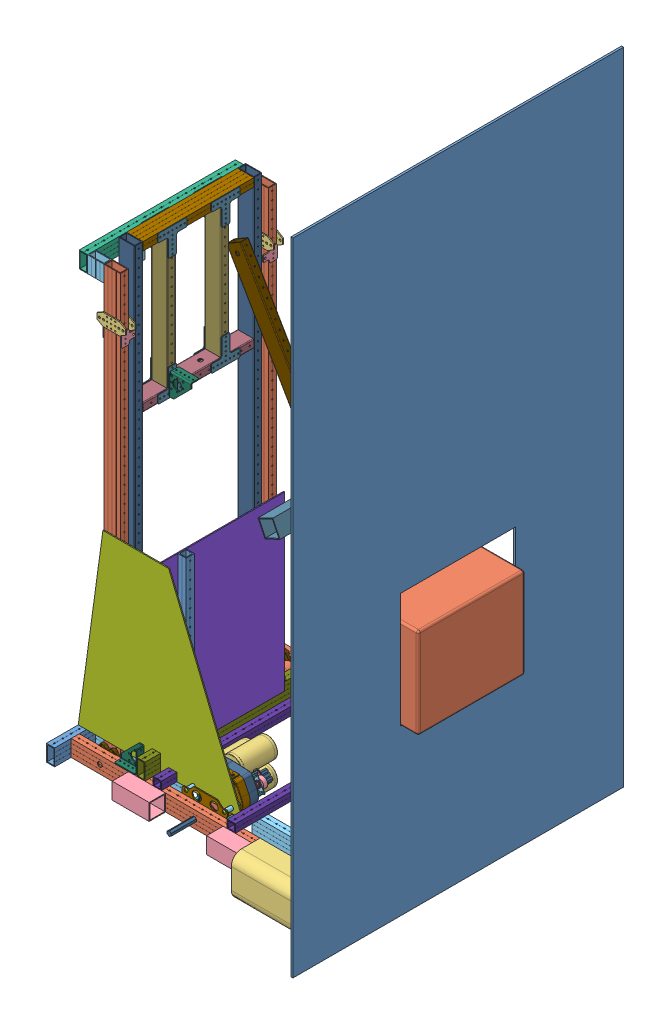
SolidWorks assembly Test Robot 3, configuration Default. Lengths in mm.
Overall size (1219.2 2133.6 1022.35).
481 component instances, 134 part files, 68 mates.
Components (placement in the parent):
- Test Base 3-1: Test Base 3 [Default] at (-213.2986 -131.6714 217.4582) size (990.6 641.86 863.6)
  - Base Rear Rail-1: Base Rear Rail [Default] at (282.1219 360.9185 104.1623) size (25.4 50.8 685.8)
  - Base Side Rail-1: Base Side Rail [Default] at (1044.1219 360.9185 789.9623) x (0 0 1) z (-1 0 0) size (25.4 50.8 762)
  - Base Side Rail-2: Base Side Rail [Default] at (1044.1219 360.9185 231.1623) x (0 0 1) z (-1 0 0) size (25.4 50.8 762)
  - Blue Bumper-1: Blue Bumper [Default] at (1171.1219 335.5185 942.3623) x (0 0 -1) z (1 0 0) size (241.3 127 241.3)
  - Blue Bumper-2: Blue Bumper [Default] at (1171.1219 335.5185 78.7623) x (-1 0 0) z (0 0 -1) size (241.3 127 241.3)
  - Bumper Support Bar-2: Bumper Support Bar [Default] at (879.0219 335.5185 166.0294) x (0 0 1) z (-1 0 0) size (50.8 50.8 114.3)
  - Bumper Support Bar-4: Bumper Support Bar [Default] at (586.9219 335.5185 166.0294) x (0 0 1) z (-1 0 0) size (50.8 50.8 114.3)
  - Bumper Support Bar-7: Bumper Support Bar [Default] at (586.9219 335.5185 801.0294) x (0 0 1) z (-1 0 0) size (50.8 50.8 114.3)
  - Bumper Support Bar-8: Bumper Support Bar [Default] at (879.0219 335.5185 801.0294) x (0 0 1) z (-1 0 0) size (50.8 50.8 114.3)
  - Base Side Rail Internal-1: Base Side Rail Internal [Default] at (-175.0781 360.9185 713.7623) x (0 0 -1) z (1 0 0) size (25.4 50.8 279.4)
  - Base Side Rail Internal-4: Base Side Rail Internal [Default] at (1044.1219 360.9185 307.3623) x (0 0 1) z (-1 0 0) size (25.4 50.8 279.4)
  - Base Front Rail-1: Base Front Rail [Default] at (1069.5219 360.9185 104.1623) size (25.4 50.8 152.4)
  - 3 CIM Ball Shifter with WCD Output-1: 3 CIM Ball Shifter with WCD Output [Default] at (711.3612 400.7203 682.3171) x (0 1 0) z (0 0 1) size (169.11 183.68 312.65)
    - 217-2733-001 Rev2-1: 217-2733-001 Rev2 [Default] at (0 53.4162 37.6682) x (0 0 1) z (-0.00054 -1 0) size (7.11 24.61 24.61)
    - 217-2733-001 Rev2-2: 217-2733-001 Rev2 [Default] at (0 53.4162 7.9248) x (0 0 -1) z (-0.038475 0.99926 0) size (7.11 24.61 24.61)
    - 217-2731-001 Rev2-1: 217-2731-001 Rev2 [Default] at (0 0 0.0381) x (-0.099212 0.995066 0) z (0.995066 0.099212 0) size (31.12 7.94 31.12)
    - 217-2789-001 Rev2-1: 217-2789-001 Rev2 [Default] at (0 0 43.2943) x (0 0 -1) z (-0.58471 0.811243 0) size (11.1 38.4 38.4)
    - 217-2778-001 Rev2_NCQ8A075-050M_1-1: 217-2778-001 Rev2_NCQ8A075-050M_1 [Default] at (0 0 -53.848) x (-0.707107 0.707107 0) z (0 0 1) size (31.75 33.34 39.88)
      - 217-2778-002_075A-1: 217-2778-002_075A [Default] at origin size (31.75 33.34 26.92)
      - 217-2778-003_075M-1: 217-2778-003_075M [Default] at (0 0 -8.85) x (0.866025 -0.5 0) z (0 0 1) size (18.95 18.95 35.27)
      - 217-2778-004_075-1: 217-2778-004_075 [Default] at (0 0 10.362) size (21 20.74 0.97)
    - 217-2428-012 Rev2-1: 217-2428-012 Rev2 [Default] at (0 0 -40.386) size (63.5 22.23 2.29)
    - 217-2428-005 Rev1-1: 217-2428-005 Rev1 [Default] at (25.4 0 -19.05) x (-0.557362 -0.83027 0) z (-0.83027 0.557362 0) size (7.33 38.98 6.35)
    - 217-2428-005 Rev1-2: 217-2428-005 Rev1 [Default] at (-25.4 0 -19.05) x (0.667436 0.744667 0) z (0.744667 -0.667436 0) size (7.33 38.98 6.35)
    - SCREW-832-0375-1: SCREW-832-0375 [Default] at (25.4 0 -42.5958) x (0 0 1) z (-0.875404 0.483392 0) size (11.73 7.92 7.92)
    - SCREW-832-0375-2: SCREW-832-0375 [Default] at (-25.4 0 -42.5958) x (0 0 1) z (-0.966319 0.257347 0) size (11.73 7.92 7.92)
    - SCREW-832-0375-3: SCREW-832-0375 [Default] at (25.4 0 5.3848) x (0 0 -1) z (1 0 0) size (11.73 7.92 7.92)
    - SCREW-832-0375-4: SCREW-832-0375 [Default] at (-25.4 0 5.3848) x (0 0 -1) z (0.941463 -0.337115 0) size (11.73 7.92 7.92)
    - SBS1_SBS-0632-0250-1: SBS1_SBS-0632-0250 [Default] at (15.494 0 -36.2458) x (0 0 -1) z (0.854303 -0.519775 0) size (8.57 6.68 6.65)
    - SBS1_SBS-0632-0250-2: SBS1_SBS-0632-0250 [Default] at (-15.494 0 -36.2458) x (0 0 -1) z (0.854303 -0.519775 0) size (8.57 6.68 6.65)
    - 217-4098-100 Rev1-1: 217-4098-100 Rev1 [Default] at (0 0 -16.927) x (-0.503316 0.864103 0) z (0 0 1) size (18.03 19.79 22.46)
      - 217-4098-006 Rev2-1: 217-4098-006 Rev2 [Default] at (0 0 -4.6312) x (0 -1 0) z (0 0 -1) size (18.09 11.02 22.46)
      - 217-4098-006 Rev2-2: 217-4098-006 Rev2 [Default] at (0 0 -4.6312) x (0 1 0) z (0 0 -1) size (18.09 11.02 22.46)
      - 217-3489-001 Rev1-1: 217-3489-001 Rev1 [Default] at (0 0 -4.6312) x (0 0 1) z (-0.980217 -0.197926 0) size (4.77 12.7 12.7)
      - 97633A130_97633A130_grv-1: 97633A130_97633A130_grv [Default] at (0 0 -7.33) x (0 0 -1) z (0.979861 0.199683 0) size (0.64 8.74 7.34)
      - 91251A107_91251A107-1: 91251A107_91251A107 [Default] at (-4.8375 -6.735 -9.4343) x (0 0.863883 -0.503692) z (-1 0 0) size (4.65 4.65 10.79)
      - 91251A107_91251A107-2: 91251A107_91251A107 [Default] at (4.8375 6.735 -9.4343) x (0 0.470889 -0.882193) z (1 0 0) size (4.65 4.65 10.79)
    - 217-2428-017 Rev2-1: 217-2428-017 Rev2 [Default] at (12.7 -21.997 -3.614) x (-0.578458 -0.815712 0) z (0 0 -1) size (14.73 14.73 7.37)
    - 217-2428-016 Rev3_Spur01-1: 217-2428-016 Rev3_Spur01 [Default] at (0 0 -3.614) x (0.873157 -0.48744 0) z (0 0 1) size (40.67 40.74 13.32)
    - 217-2428-019 Rev1-1: 217-2428-019 Rev1 [Default] at (12.7 -21.997 -20.6248) x (0.866025 0.5 0) z (0 0 1) size (50.8 19.05 1.57)
    - 217-2428-006 Rev1-1: 217-2428-006 Rev1 [Default] at (32.079 -14.2875 -9.525) x (-0.752416 0.658689 0) z (0.658689 0.752416 0) size (7.33 19.93 6.35)
    - 217-2428-006 Rev1-2: 217-2428-006 Rev1 [Default] at (-3.6662 -34.925 -9.525) x (0.84498 0.534798 0) z (0.534798 -0.84498 0) size (7.33 19.93 6.35)
    - SCREW-832-0375-5: SCREW-832-0375 [Default] at (32.079 -14.2875 4.7498) x (0 0 -1) z (0.980613 0.195955 0) size (11.73 7.92 7.92)
    - SCREW-832-0375-6: SCREW-832-0375 [Default] at (-3.6662 -34.925 5.3848) x (0 0 -1) z (-0.672515 -0.740083 0) size (11.73 7.92 7.92)
    - SCREW-832-0375-7: SCREW-832-0375 [Default] at (-3.6662 -34.925 -22.8346) x (0 0 1) z (0.948865 0.315681 0) size (11.73 7.92 7.92)
    - SCREW-832-0375-8: SCREW-832-0375 [Default] at (32.079 -14.2875 -22.8346) x (0 0 1) z (-0.875404 0.483392 0) size (11.73 7.92 7.92)
    - 217-2614-001_12t-1: 217-2614-001_12t [Default] at (36.9798 39.6868 15.8623) x (-0.087156 0.996195 0) z (0 0 1) size (18.29 18.29 19)
    - 217-2761-001 rev1-1: 217-2761-001 rev1 [Default] at (33.1943 39.3556 16.1) x (0.087156 -0.996195 0) z (0 0 1) size (2 2 20)
    - 217-2761-001 rev1-2: 217-2761-001 rev1 [Default] at (-40.7653 40.018 16.1) x (0.087156 0.996195 0) z (0 0 1) size (2 2 20)
    - 217-2614-001_12t-2: 217-2614-001_12t [Default] at (-36.9798 39.6868 15.8623) x (0.087156 0.996195 0) z (0 0 1) size (18.29 18.29 19)
    - 217-2614-001_12t-3: 217-2614-001_12t [Default] at (0 92.8624 15.8623) x (0.97459 0.223996 0) z (0 0 1) size (18.29 18.29 19)
    - 217-2761-001 rev1-3: 217-2761-001 rev1 [Default] at (-0.8512 96.5658 16.1) x (0.97459 0.223996 0) z (0 0 1) size (2 2 20)
    - 217-3195-002 rev2-1: 217-3195-002 rev2 [Default] at (0 0 50.546) x (-1 0 0) z (0 0 -1) size (114.31 152.24 24.96)
    - 217-3195-001 Rev1-1: 217-3195-001 Rev1 [Default] at origin size (113.41 152.24 26.86)
    - Nylock Nut_NNY2520-ZC-1: Nylock Nut_NNY2520-ZC [Default] at (48.8823 73.025 37.846) x (0 0.866025 -0.5) z (-1 0 0) size (12.85 11.89 7.62)
    - Nylock Nut_NNY2520-ZC-2: Nylock Nut_NNY2520-ZC [Default] at (48.8823 -3.175 37.846) x (0 0 -1) z (-1 0 0) size (12.85 11.89 7.62)
    - Nylock Nut_NNY2520-ZC-3: Nylock Nut_NNY2520-ZC [Default] at (44.45 85.725 7.8613) x (0 1 0) z (0 0 -1) size (12.85 11.89 7.62)
    - 276-1027-001-1: 276-1027-001 [Default] at (47.625 58.1787 6.35) x (0 1 0) z (-1 0 0) size (8.61 5.64 9.94)
    - 276-1027-001-2: 276-1027-001 [Default] at (-47.625 58.1787 6.35) x (0 -1 0) z (1 0 0) size (8.61 5.64 9.94)
    - SCREW-832-1750-1: SCREW-832-1750 [Default] at (-47.625 58.1787 47.0408) x (0 0 -1) z (-0.960822 -0.277167 0) size (46.66 7.92 7.92)
    - SCREW-832-1750-2: SCREW-832-1750 [Default] at (47.625 58.1787 47.0408) x (0 0 -1) z (-0.960822 -0.277167 0) size (46.66 7.92 7.92)
    - Nylock Nut_NNY2520-ZC-4: Nylock Nut_NNY2520-ZC [Default] at (44.45 -15.875 7.8613) x (0 1 0) z (0 0 -1) size (12.85 11.89 7.62)
    - 217-2428-004 Rev3-1: 217-2428-004 Rev3 [Default] at (0 53.4162 22.7711) x (-0.709585 0.70462 0) z (0 0 1) size (11 9.53 43.92)
    - SBS1_SBS-2520-1625SS-1: SBS1_SBS-2520-1625SS [Default] at (44.45 85.725 42.4688) x (0 0 -1) z (-0.251219 0.96793 0) size (45.3 11.2 11.18)
    - SBS1_SBS-2520-1625SS-2: SBS1_SBS-2520-1625SS [Default] at (44.45 -15.875 42.4688) x (0 0 -1) z (-0.251219 0.96793 0) size (45.3 11.2 11.18)
    - SBS1_SBS2520-1750-1: SBS1_SBS2520-1750 [Default] at (-44.45 85.725 7.4422) x (0 0 1) z (-0.031478 0.999504 0) size (48.48 11.22 11.17)
    - SBS1_SBS2520-1750-2: SBS1_SBS2520-1750 [Default] at (-44.45 -15.875 7.4422) x (0 0 1) z (-0.937114 -0.349025 0) size (48.48 11.22 11.17)
    - 217-2428-021 Rev1-1: 217-2428-021 Rev1 [Default] at (0 53.4162 9.5123) x (0.451333 -0.892356 0) z (0 0 1) size (15.88 15.88 3.17)
    - 217-2428-029 Rev1-1: 217-2428-029 Rev1 [Default] at (0 53.4162 36.957) x (0.999846 0.017557 0) z (0 0 1) size (15.88 15.88 1.12)
    - Grayhill Lock Washer-1: Grayhill Lock Washer [Default] at (12.7 -21.997 -18.6817) x (0.467173 -0.884166 0) z (0 0 1) size (19.69 19.69 0.74)
    - Grayhill Nut-1: Grayhill Nut [Default] at (12.7 -21.997 -17.0434) x (0.984088 0.177684 0) z (0 0 1) size (18.33 15.88 2.54)
    - 217-2000-1: 217-2000 [Default] at (0 92.8624 0) x (0 0 -1) z (0.223996 -0.97459 0) size (150.2 64.01 64.01)
    - 217-2000-2: 217-2000 [Default] at (-36.9798 39.6868 0) x (0 0 -1) z (0.996195 -0.087156 0) size (150.2 64.01 64.01)
    - 217-2000-3: 217-2000 [Default] at (36.9798 39.6868 0) x (0 0 -1) z (0.996195 0.087156 0) size (150.2 64.01 64.01)
    - Grahill Encoder-1: Grahill Encoder [Default] at (12.7 -21.997 -16.1798) x (-0.580071 0.814566 0) z (-0.814566 -0.580071 0) size (31.75 31.12 31.75)
    - 217-3195-009 Rev1_wcd 2-1: 217-3195-009 Rev1_wcd 2 [Default] at (0 85.725 50.546) x (-0.998427 -0.056065 0) z (0 0 1) size (12.7 12.7 41.27)
    - 217-3195-006 Rev1_WCD-1: 217-3195-006 Rev1_WCD [Default] at (-44.45 85.725 44.1452) x (0.5 0.866025 0) z (0 0 1) size (12.7 14.66 47.62)
    - 217-3195-009 Rev1_wcd 2-2: 217-3195-009 Rev1_wcd 2 [Default] at (0 -31.75 50.546) x (0.947633 0.319361 0) z (0 0 1) size (12.7 12.7 41.27)
    - 217-3195-006 Rev1_WCD-2: 217-3195-006 Rev1_WCD [Default] at (-44.45 -15.875 44.1452) x (0.5 -0.866025 0) z (0 0 1) size (12.7 14.66 47.62)
    - Nylock Nut_NNY2520-ZC-5: Nylock Nut_NNY2520-ZC [Default] at (0 -31.75 45.0723) x (-0.5 0.866025 0) z (0 0 -1) size (12.85 11.89 7.62)
    - Nylock Nut_NNY2520-ZC-6: Nylock Nut_NNY2520-ZC [Default] at (0 85.725 45.0723) x (-0.5 0.866025 0) z (0 0 -1) size (12.85 11.89 7.62)
    - SBS1_SBS-2520-2250-1: SBS1_SBS-2520-2250 [Default] at (0 -31.75 98.298) x (0 0 -1) z (-0.933488 -0.358607 0) size (61.18 11.22 11.17)
    - SBS1_SBS2520-0625ZC-1: SBS1_SBS2520-0625ZC [Default] at (-44.45 85.725 98.298) x (0 0 -1) z (0.400817 0.916158 0) size (19.57 11.22 11.17)
    - SBS1_SBS2520-0625ZC-2: SBS1_SBS2520-0625ZC [Default] at (-44.45 -15.875 98.298) x (0 0 -1) z (-0.75178 -0.659414 0) size (19.57 11.22 11.17)
    - SBS1_SBS-2520-2250-2: SBS1_SBS-2520-2250 [Default] at (0 85.725 98.298) x (0 0 -1) z (0.056677 -0.998393 0) size (61.18 11.22 11.17)
    - 217-3195-003 rev2-1: 217-3195-003 rev2 [Default] at (0 0 94.9452) size (88.62 139.7 3.17)
    - 217-2617-003 Rev1-1: 217-2617-003 Rev1 [Default] at (-39.878 35.5392 121.8535) x (-0.5 -0.866025 0) z (0 0 1) size (14.66 12.7 152.4)
    - 217-3109-001 Rev1-1: 217-3109-001 Rev1 [Default] at (-39.878 35.5392 49.1808) x (0 0 1) z (0.312889 -0.94979 0) size (7.94 28.57 28.57)
    - 217-2734-001 Rev3-1: 217-2734-001 Rev3 [Default] at (-39.878 35.5392 98.1202) x (1 0 0) z (0 1 0) size (31.12 7.94 31.12)
    - 217-2617-004 Rev1_97431A340_grv-1: 217-2617-004 Rev1_97431A340_grv [Default] at (-39.878 35.5392 54.8961) x (0 0 1) z (-0.124043 -0.992277 0) size (1.07 20.42 18.58)
    - 217-2617-004 Rev1_97431A340_grv-2: 217-2617-004 Rev1_97431A340_grv [Default] at (0 0 69.215) x (0 0 1) z (-0.124043 -0.992277 0) size (1.07 20.42 18.58)
    - 217-2702-001_20t-1: 217-2702-001_20t [Default] at (0 0 62.357) x (0.998435 0.055929 0) z (0 0 1) size (28.2 28.2 12.65)
    - 217-2715-002 Rev1_64t-1: 217-2715-002 Rev1_64t [Default] at (-39.878 35.5392 61.7541) x (0.866025 -0.5 0) z (0 0 1) size (84.3 84.3 12.65)
    - 217-2704-001_24-1: 217-2704-001_24 [Default] at (0 0 62.357) x (0.450781 0.892635 0) z (0 0 -1) size (33.29 33.29 12.65)
    - 217-2714-002 Rev1_60t-1: 217-2714-002 Rev1_60t [Default] at (-39.878 35.5392 61.7541) x (0.866025 -0.5 0) z (0 0 1) size (78.95 78.95 12.65)
    - 217-3221-002 Rev1-1: 217-3221-002 Rev1 [Default] at (-39.878 35.5392 61.7414) x (0 -1 0) z (0 0 1) size (71.39 71.45 12.62)
    - 217-2705-001_30t-1: 217-2705-001_30t [Default] at (0 0 62.357) x (0.547654 -0.836705 0) z (0 0 1) size (41.01 41.12 12.65)
    - 217-2712-002 Rev1_50t-1: 217-2712-002 Rev1_50t [Default] at (-39.878 35.5392 61.7541) x (0.866025 -0.5 0) z (0 0 1) size (66.7 66.76 12.65)
    - 217-2706-001_34t-1: 217-2706-001_34t [Default] at (0 0 62.357) x (0.998435 0.055929 0) z (0 0 1) size (46.46 46.56 12.65)
    - 217-3288-001 Rev3-1: 217-3288-001 Rev3 [Default] at (0 0 0.0889) x (0.055929 -0.998435 0) z (0 0 1) size (99.51 99.53 98.3)
      - 217-2428-008 Rev2-1: 217-2428-008 Rev2 [Default] at (0 0 10.2679) size (31.75 31.75 1.59)
      - 217-2428-028 Rev1_97633A250-1: 217-2428-028 Rev1_97633A250 [Default] at (0 0 37.1221) x (0 0 1) z (0.9357 -0.352797 0) size (1.07 23.39 21.18)
      - 217-4099-000 Rev2_high gear-1: 217-4099-000 Rev2_high gear [Default] x (-1 0 0) z (0 0 1) size (22.23 22.23 98.3)
        - 217-4098-005 Rev1_91612A226-1: 217-4098-005 Rev1_91612A226 [Default] at (0 0 46.2661) x (-0.144757 0 0.989467) z (0 -1 0) size (3.02 3.15 18.22)
        - 217-4098-003 Rev2-1: 217-4098-003 Rev2 [Default] x (1 0 0) z (0 0 -1) size (22.23 22.23 55.94)
        - 217-4099-002 Rev3-1: 217-4099-002 Rev3 [Default] at (0 0 53.467) x (0 0 1) z (-1 0 0) size (40.96 12.73 14.67)
        - 217-4098-004 Rev1-1: 217-4098-004 Rev1 [Default] at (0 0 14.2494) x (0.393904 0.919152 0) z (0 0 1) size (11.68 11.68 56)
      - 217-2428-007 Rev1-1: 217-2428-007 Rev1 [Default] at (7.809 4.5085 14.2494) x (-0.69071 0.455693 -0.561483) z (-0.67559 -0.683536 0.276329) size (6.35 6.35 6.35)
      - 217-2428-007 Rev1-2: 217-2428-007 Rev1 [Default] at (5.4343 3.1375 26.9494) x (-0.162331 -0.978398 0.128005) z (0.857281 -0.204076 -0.472676) size (6.35 6.35 6.35)
      - 217-3212-101 Rev1-1: 217-3212-101 Rev1 [Default] at (-11.5751 10.4131 45.3224) x (0.923728 0.383049 0) z (0 0 -1) size (46.46 46.56 12.7)
        - 217-2428-022 Rev1-1: 217-2428-022 Rev1 [Default] at (6.7035 14.0527 24.6087) size (28.57 28.57 6.1)
        - 217-3212-001 Rev1_34t-1: 217-3212-001 Rev1_34t [Default] at (6.7035 14.0527 27.9107) size (46.46 46.56 11.11)
      - 217-3222-101 Rev1-1: 217-3222-101 Rev1 [Default] at (21.0941 -5.2804 52.7371) x (-0.889163 -0.457591 0) z (0 0 -1) size (73.87 73.92 12.7)
        - 217-2428-022 Rev1-1: 217-2428-022 Rev1 [Default] at (16.3398 14.3476 19.3234) size (28.57 28.57 6.1)
        - 217-3222-001 Rev1_Spur01-1: 217-3222-001 Rev1_Spur01 [Default] at (16.3398 14.3476 22.6254) x (0.999377 0.0353 0) z (0 0 1) size (71.39 71.45 11.11)
      - 217-2428-007 Rev1-3: 217-2428-007 Rev1 [Default] at (-5.4343 3.1375 26.9494) x (0.928483 0.348617 0.128005) z (-0.251905 0.844465 -0.472676) size (6.35 6.35 6.35)
      - 217-2428-007 Rev1-4: 217-2428-007 Rev1 [Default] at (0 -6.275 26.9494) x (-0.766153 0.629782 0.128005) z (-0.605376 -0.640389 -0.472676) size (6.35 6.35 6.35)
      - 217-2428-007 Rev1-5: 217-2428-007 Rev1 [Default] at (-7.809 4.5085 14.2494) x (-0.049287 -0.826019 -0.561483) z (0.929754 -0.24331 0.276329) size (6.35 6.35 6.35)
      - 217-2428-007 Rev1-6: 217-2428-007 Rev1 [Default] at (0 -9.017 14.2494) x (0.739997 0.370326 -0.561483) z (-0.254164 0.926846 0.276329) size (6.35 6.35 6.35)
    - 217-3210-001 Rev1_30t-1: 217-3210-001 Rev1_30t [Default] at (0 53.4162 30.0736) x (-0.966828 0.255427 0) z (0 0 1) size (41.01 41.12 12.65)
    - 217-2711-002 Rev1_50t-1: 217-2711-002 Rev1_50t [Default] at (0 53.4162 17.4244) x (0.262208 -0.965011 0) z (0 0 1) size (66.7 66.76 12.65)
  - 3 CIM Ball Shifter with WCD Output-2: 3 CIM Ball Shifter with WCD Output [Default] at (640.2827 400.7203 338.8075) x (0 1 0) z (0 0 -1) size (169.11 183.68 312.65)
    - 217-2733-001 Rev2-1: 217-2733-001 Rev2 [Default] at (0 53.4162 37.6682) x (0 0 1) z (-0.00054 -1 0) size (7.11 24.61 24.61)
    - 217-2733-001 Rev2-2: 217-2733-001 Rev2 [Default] at (0 53.4162 7.9248) x (0 0 -1) z (-0.038475 0.99926 0) size (7.11 24.61 24.61)
    - 217-2731-001 Rev2-1: 217-2731-001 Rev2 [Default] at (0 0 0.0381) x (-0.099212 0.995066 0) z (0.995066 0.099212 0) size (31.12 7.94 31.12)
    - 217-2789-001 Rev2-1: 217-2789-001 Rev2 [Default] at (0 0 43.2943) x (0 0 -1) z (-0.58471 0.811243 0) size (11.1 38.4 38.4)
    - 217-2778-001 Rev2_NCQ8A075-050M_1-1: 217-2778-001 Rev2_NCQ8A075-050M_1 [Default] at (0 0 -53.848) x (-0.707107 0.707107 0) z (0 0 1) size (31.75 33.34 39.88)
      - 217-2778-002_075A-1: 217-2778-002_075A [Default] at origin size (31.75 33.34 26.92)
      - 217-2778-003_075M-1: 217-2778-003_075M [Default] at (0 0 -8.85) x (0.866025 -0.5 0) z (0 0 1) size (18.95 18.95 35.27)
      - 217-2778-004_075-1: 217-2778-004_075 [Default] at (0 0 10.362) size (21 20.74 0.97)
    - 217-2428-012 Rev2-1: 217-2428-012 Rev2 [Default] at (0 0 -40.386) size (63.5 22.23 2.29)
    - 217-2428-005 Rev1-1: 217-2428-005 Rev1 [Default] at (25.4 0 -19.05) x (-0.557362 -0.83027 0) z (-0.83027 0.557362 0) size (7.33 38.98 6.35)
    - 217-2428-005 Rev1-2: 217-2428-005 Rev1 [Default] at (-25.4 0 -19.05) x (0.667436 0.744667 0) z (0.744667 -0.667436 0) size (7.33 38.98 6.35)
    - SCREW-832-0375-1: SCREW-832-0375 [Default] at (25.4 0 -42.5958) x (0 0 1) z (-0.875404 0.483392 0) size (11.73 7.92 7.92)
    - SCREW-832-0375-2: SCREW-832-0375 [Default] at (-25.4 0 -42.5958) x (0 0 1) z (-0.966319 0.257347 0) size (11.73 7.92 7.92)
    - SCREW-832-0375-3: SCREW-832-0375 [Default] at (25.4 0 5.3848) x (0 0 -1) z (1 0 0) size (11.73 7.92 7.92)
    - SCREW-832-0375-4: SCREW-832-0375 [Default] at (-25.4 0 5.3848) x (0 0 -1) z (0.941463 -0.337115 0) size (11.73 7.92 7.92)
    - SBS1_SBS-0632-0250-1: SBS1_SBS-0632-0250 [Default] at (15.494 0 -36.2458) x (0 0 -1) z (0.854303 -0.519775 0) size (8.57 6.68 6.65)
    - SBS1_SBS-0632-0250-2: SBS1_SBS-0632-0250 [Default] at (-15.494 0 -36.2458) x (0 0 -1) z (0.854303 -0.519775 0) size (8.57 6.68 6.65)
    - 217-4098-100 Rev1-1: 217-4098-100 Rev1 [Default] at (0 0 -16.927) x (-0.503316 0.864103 0) z (0 0 1) size (18.03 19.79 22.46)
      - 217-4098-006 Rev2-1: 217-4098-006 Rev2 [Default] at (0 0 -4.6312) x (0 -1 0) z (0 0 -1) size (18.09 11.02 22.46)
      - 217-4098-006 Rev2-2: 217-4098-006 Rev2 [Default] at (0 0 -4.6312) x (0 1 0) z (0 0 -1) size (18.09 11.02 22.46)
      - 217-3489-001 Rev1-1: 217-3489-001 Rev1 [Default] at (0 0 -4.6312) x (0 0 1) z (-0.980217 -0.197926 0) size (4.77 12.7 12.7)
      - 97633A130_97633A130_grv-1: 97633A130_97633A130_grv [Default] at (0 0 -7.33) x (0 0 -1) z (0.979861 0.199683 0) size (0.64 8.74 7.34)
      - 91251A107_91251A107-1: 91251A107_91251A107 [Default] at (-4.8375 -6.735 -9.4343) x (0 0.863883 -0.503692) z (-1 0 0) size (4.65 4.65 10.79)
      - 91251A107_91251A107-2: 91251A107_91251A107 [Default] at (4.8375 6.735 -9.4343) x (0 0.470889 -0.882193) z (1 0 0) size (4.65 4.65 10.79)
    - 217-2428-017 Rev2-1: 217-2428-017 Rev2 [Default] at (12.7 -21.997 -3.614) x (-0.578458 -0.815712 0) z (0 0 -1) size (14.73 14.73 7.37)
    - 217-2428-016 Rev3_Spur01-1: 217-2428-016 Rev3_Spur01 [Default] at (0 0 -3.614) x (0.873157 -0.48744 0) z (0 0 1) size (40.67 40.74 13.32)
    - 217-2428-019 Rev1-1: 217-2428-019 Rev1 [Default] at (12.7 -21.997 -20.6248) x (0.866025 0.5 0) z (0 0 1) size (50.8 19.05 1.57)
    - 217-2428-006 Rev1-1: 217-2428-006 Rev1 [Default] at (32.079 -14.2875 -9.525) x (-0.752416 0.658689 0) z (0.658689 0.752416 0) size (7.33 19.93 6.35)
    - 217-2428-006 Rev1-2: 217-2428-006 Rev1 [Default] at (-3.6662 -34.925 -9.525) x (0.84498 0.534798 0) z (0.534798 -0.84498 0) size (7.33 19.93 6.35)
    - SCREW-832-0375-5: SCREW-832-0375 [Default] at (32.079 -14.2875 4.7498) x (0 0 -1) z (0.980613 0.195955 0) size (11.73 7.92 7.92)
    - SCREW-832-0375-6: SCREW-832-0375 [Default] at (-3.6662 -34.925 5.3848) x (0 0 -1) z (-0.672515 -0.740083 0) size (11.73 7.92 7.92)
    - SCREW-832-0375-7: SCREW-832-0375 [Default] at (-3.6662 -34.925 -22.8346) x (0 0 1) z (0.948865 0.315681 0) size (11.73 7.92 7.92)
    - SCREW-832-0375-8: SCREW-832-0375 [Default] at (32.079 -14.2875 -22.8346) x (0 0 1) z (-0.875404 0.483392 0) size (11.73 7.92 7.92)
    - 217-2614-001_12t-1: 217-2614-001_12t [Default] at (36.9798 39.6868 15.8623) x (-0.087156 0.996195 0) z (0 0 1) size (18.29 18.29 19)
    - 217-2761-001 rev1-1: 217-2761-001 rev1 [Default] at (33.1943 39.3556 16.1) x (0.087156 -0.996195 0) z (0 0 1) size (2 2 20)
    - 217-2761-001 rev1-2: 217-2761-001 rev1 [Default] at (-40.7653 40.018 16.1) x (0.087156 0.996195 0) z (0 0 1) size (2 2 20)
    - 217-2614-001_12t-2: 217-2614-001_12t [Default] at (-36.9798 39.6868 15.8623) x (0.087156 0.996195 0) z (0 0 1) size (18.29 18.29 19)
    - 217-2614-001_12t-3: 217-2614-001_12t [Default] at (0 92.8624 15.8623) x (0.97459 0.223996 0) z (0 0 1) size (18.29 18.29 19)
    - 217-2761-001 rev1-3: 217-2761-001 rev1 [Default] at (-0.8512 96.5658 16.1) x (0.97459 0.223996 0) z (0 0 1) size (2 2 20)
    - 217-3195-002 rev2-1: 217-3195-002 rev2 [Default] at (0 0 50.546) x (-1 0 0) z (0 0 -1) size (114.31 152.24 24.96)
    - 217-3195-001 Rev1-1: 217-3195-001 Rev1 [Default] at origin size (113.41 152.24 26.86)
    - Nylock Nut_NNY2520-ZC-1: Nylock Nut_NNY2520-ZC [Default] at (48.8823 73.025 37.846) x (0 0.866025 -0.5) z (-1 0 0) size (12.85 11.89 7.62)
    - Nylock Nut_NNY2520-ZC-2: Nylock Nut_NNY2520-ZC [Default] at (48.8823 -3.175 37.846) x (0 0 -1) z (-1 0 0) size (12.85 11.89 7.62)
    - Nylock Nut_NNY2520-ZC-3: Nylock Nut_NNY2520-ZC [Default] at (44.45 85.725 7.8613) x (0 1 0) z (0 0 -1) size (12.85 11.89 7.62)
    - 276-1027-001-1: 276-1027-001 [Default] at (47.625 58.1787 6.35) x (0 1 0) z (-1 0 0) size (8.61 5.64 9.94)
    - 276-1027-001-2: 276-1027-001 [Default] at (-47.625 58.1787 6.35) x (0 -1 0) z (1 0 0) size (8.61 5.64 9.94)
    - SCREW-832-1750-1: SCREW-832-1750 [Default] at (-47.625 58.1787 47.0408) x (0 0 -1) z (-0.960822 -0.277167 0) size (46.66 7.92 7.92)
    - SCREW-832-1750-2: SCREW-832-1750 [Default] at (47.625 58.1787 47.0408) x (0 0 -1) z (-0.960822 -0.277167 0) size (46.66 7.92 7.92)
    - Nylock Nut_NNY2520-ZC-4: Nylock Nut_NNY2520-ZC [Default] at (44.45 -15.875 7.8613) x (0 1 0) z (0 0 -1) size (12.85 11.89 7.62)
    - 217-2428-004 Rev3-1: 217-2428-004 Rev3 [Default] at (0 53.4162 22.7711) x (-0.709585 0.70462 0) z (0 0 1) size (11 9.53 43.92)
    - SBS1_SBS-2520-1625SS-1: SBS1_SBS-2520-1625SS [Default] at (44.45 85.725 42.4688) x (0 0 -1) z (-0.251219 0.96793 0) size (45.3 11.2 11.18)
    - SBS1_SBS-2520-1625SS-2: SBS1_SBS-2520-1625SS [Default] at (44.45 -15.875 42.4688) x (0 0 -1) z (-0.251219 0.96793 0) size (45.3 11.2 11.18)
    - SBS1_SBS2520-1750-1: SBS1_SBS2520-1750 [Default] at (-44.45 85.725 7.4422) x (0 0 1) z (-0.031478 0.999504 0) size (48.48 11.22 11.17)
    - SBS1_SBS2520-1750-2: SBS1_SBS2520-1750 [Default] at (-44.45 -15.875 7.4422) x (0 0 1) z (-0.937114 -0.349025 0) size (48.48 11.22 11.17)
    - 217-2428-021 Rev1-1: 217-2428-021 Rev1 [Default] at (0 53.4162 9.5123) x (0.451333 -0.892356 0) z (0 0 1) size (15.88 15.88 3.17)
    - 217-2428-029 Rev1-1: 217-2428-029 Rev1 [Default] at (0 53.4162 36.957) x (0.999846 0.017557 0) z (0 0 1) size (15.88 15.88 1.12)
    - Grayhill Lock Washer-1: Grayhill Lock Washer [Default] at (12.7 -21.997 -18.6817) x (0.467173 -0.884166 0) z (0 0 1) size (19.69 19.69 0.74)
    - Grayhill Nut-1: Grayhill Nut [Default] at (12.7 -21.997 -17.0434) x (0.984088 0.177684 0) z (0 0 1) size (18.33 15.88 2.54)
    - 217-2000-1: 217-2000 [Default] at (0 92.8624 0) x (0 0 -1) z (0.223996 -0.97459 0) size (150.2 64.01 64.01)
    - 217-2000-2: 217-2000 [Default] at (-36.9798 39.6868 0) x (0 0 -1) z (0.996195 -0.087156 0) size (150.2 64.01 64.01)
    - 217-2000-3: 217-2000 [Default] at (36.9798 39.6868 0) x (0 0 -1) z (0.996195 0.087156 0) size (150.2 64.01 64.01)
    - Grahill Encoder-1: Grahill Encoder [Default] at (12.7 -21.997 -16.1798) x (-0.580071 0.814566 0) z (-0.814566 -0.580071 0) size (31.75 31.12 31.75)
    - 217-3195-009 Rev1_wcd 2-1: 217-3195-009 Rev1_wcd 2 [Default] at (0 85.725 50.546) x (-0.998427 -0.056065 0) z (0 0 1) size (12.7 12.7 41.27)
    - 217-3195-006 Rev1_WCD-1: 217-3195-006 Rev1_WCD [Default] at (-44.45 85.725 44.1452) x (0.5 0.866025 0) z (0 0 1) size (12.7 14.66 47.62)
    - 217-3195-009 Rev1_wcd 2-2: 217-3195-009 Rev1_wcd 2 [Default] at (0 -31.75 50.546) x (0.947633 0.319361 0) z (0 0 1) size (12.7 12.7 41.27)
    - 217-3195-006 Rev1_WCD-2: 217-3195-006 Rev1_WCD [Default] at (-44.45 -15.875 44.1452) x (0.5 -0.866025 0) z (0 0 1) size (12.7 14.66 47.62)
    - Nylock Nut_NNY2520-ZC-5: Nylock Nut_NNY2520-ZC [Default] at (0 -31.75 45.0723) x (-0.5 0.866025 0) z (0 0 -1) size (12.85 11.89 7.62)
    - Nylock Nut_NNY2520-ZC-6: Nylock Nut_NNY2520-ZC [Default] at (0 85.725 45.0723) x (-0.5 0.866025 0) z (0 0 -1) size (12.85 11.89 7.62)
    - SBS1_SBS-2520-2250-1: SBS1_SBS-2520-2250 [Default] at (0 -31.75 98.298) x (0 0 -1) z (-0.933488 -0.358607 0) size (61.18 11.22 11.17)
    - SBS1_SBS2520-0625ZC-1: SBS1_SBS2520-0625ZC [Default] at (-44.45 85.725 98.298) x (0 0 -1) z (0.400817 0.916158 0) size (19.57 11.22 11.17)
    - SBS1_SBS2520-0625ZC-2: SBS1_SBS2520-0625ZC [Default] at (-44.45 -15.875 98.298) x (0 0 -1) z (-0.75178 -0.659414 0) size (19.57 11.22 11.17)
    - SBS1_SBS-2520-2250-2: SBS1_SBS-2520-2250 [Default] at (0 85.725 98.298) x (0 0 -1) z (0.056677 -0.998393 0) size (61.18 11.22 11.17)
    - 217-3195-003 rev2-1: 217-3195-003 rev2 [Default] at (0 0 94.9452) size (88.62 139.7 3.17)
    - 217-2617-003 Rev1-1: 217-2617-003 Rev1 [Default] at (-39.878 35.5392 121.8535) x (-0.5 -0.866025 0) z (0 0 1) size (14.66 12.7 152.4)
    - 217-3109-001 Rev1-1: 217-3109-001 Rev1 [Default] at (-39.878 35.5392 49.1808) x (0 0 1) z (0.312889 -0.94979 0) size (7.94 28.57 28.57)
    - 217-2734-001 Rev3-1: 217-2734-001 Rev3 [Default] at (-39.878 35.5392 98.1202) x (1 0 0) z (0 1 0) size (31.12 7.94 31.12)
    - 217-2617-004 Rev1_97431A340_grv-1: 217-2617-004 Rev1_97431A340_grv [Default] at (-39.878 35.5392 54.8961) x (0 0 1) z (-0.124043 -0.992277 0) size (1.07 20.42 18.58)
    - 217-2617-004 Rev1_97431A340_grv-2: 217-2617-004 Rev1_97431A340_grv [Default] at (0 0 69.215) x (0 0 1) z (-0.124043 -0.992277 0) size (1.07 20.42 18.58)
    - 217-2702-001_20t-1: 217-2702-001_20t [Default] at (0 0 62.357) x (0.998435 0.055929 0) z (0 0 1) size (28.2 28.2 12.65)
    - 217-2715-002 Rev1_64t-1: 217-2715-002 Rev1_64t [Default] at (-39.878 35.5392 61.7541) x (0.866025 -0.5 0) z (0 0 1) size (84.3 84.3 12.65)
    - 217-2704-001_24-1: 217-2704-001_24 [Default] at (0 0 62.357) x (0.450781 0.892635 0) z (0 0 -1) size (33.29 33.29 12.65)
    - 217-2714-002 Rev1_60t-1: 217-2714-002 Rev1_60t [Default] at (-39.878 35.5392 61.7541) x (0.866025 -0.5 0) z (0 0 1) size (78.95 78.95 12.65)
    - 217-3221-002 Rev1-1: 217-3221-002 Rev1 [Default] at (-39.878 35.5392 61.7414) x (0 -1 0) z (0 0 1) size (71.39 71.45 12.62)
    - 217-2705-001_30t-1: 217-2705-001_30t [Default] at (0 0 62.357) x (0.547654 -0.836705 0) z (0 0 1) size (41.01 41.12 12.65)
    - 217-2712-002 Rev1_50t-1: 217-2712-002 Rev1_50t [Default] at (-39.878 35.5392 61.7541) x (0.866025 -0.5 0) z (0 0 1) size (66.7 66.76 12.65)
    - 217-2706-001_34t-1: 217-2706-001_34t [Default] at (0 0 62.357) x (0.998435 0.055929 0) z (0 0 1) size (46.46 46.56 12.65)
    - 217-3288-001 Rev3-1: 217-3288-001 Rev3 [Default] at (0 0 0.0889) x (0.055929 -0.998435 0) z (0 0 1) size (99.51 99.53 98.3)
      - 217-2428-008 Rev2-1: 217-2428-008 Rev2 [Default] at (0 0 10.2679) size (31.75 31.75 1.59)
      - 217-2428-028 Rev1_97633A250-1: 217-2428-028 Rev1_97633A250 [Default] at (0 0 37.1221) x (0 0 1) z (0.9357 -0.352797 0) size (1.07 23.39 21.18)
      - 217-4099-000 Rev2_high gear-1: 217-4099-000 Rev2_high gear [Default] x (-1 0 0) z (0 0 1) size (22.23 22.23 98.3)
        - 217-4098-005 Rev1_91612A226-1: 217-4098-005 Rev1_91612A226 [Default] at (0 0 46.2661) x (-0.144757 0 0.989467) z (0 -1 0) size (3.02 3.15 18.22)
        - 217-4098-003 Rev2-1: 217-4098-003 Rev2 [Default] x (1 0 0) z (0 0 -1) size (22.23 22.23 55.94)
        - 217-4099-002 Rev3-1: 217-4099-002 Rev3 [Default] at (0 0 53.467) x (0 0 1) z (-1 0 0) size (40.96 12.73 14.67)
        - 217-4098-004 Rev1-1: 217-4098-004 Rev1 [Default] at (0 0 14.2494) x (0.393904 0.919152 0) z (0 0 1) size (11.68 11.68 56)
      - 217-2428-007 Rev1-1: 217-2428-007 Rev1 [Default] at (7.809 4.5085 14.2494) x (-0.69071 0.455693 -0.561483) z (-0.67559 -0.683536 0.276329) size (6.35 6.35 6.35)
      - 217-2428-007 Rev1-2: 217-2428-007 Rev1 [Default] at (5.4343 3.1375 26.9494) x (-0.162331 -0.978398 0.128005) z (0.857281 -0.204076 -0.472676) size (6.35 6.35 6.35)
      - 217-3212-101 Rev1-1: 217-3212-101 Rev1 [Default] at (-11.5751 10.4131 45.3224) x (0.923728 0.383049 0) z (0 0 -1) size (46.46 46.56 12.7)
        - 217-2428-022 Rev1-1: 217-2428-022 Rev1 [Default] at (6.7035 14.0527 24.6087) size (28.57 28.57 6.1)
        - 217-3212-001 Rev1_34t-1: 217-3212-001 Rev1_34t [Default] at (6.7035 14.0527 27.9107) size (46.46 46.56 11.11)
      - 217-3222-101 Rev1-1: 217-3222-101 Rev1 [Default] at (21.0941 -5.2804 52.7371) x (-0.889163 -0.457591 0) z (0 0 -1) size (73.87 73.92 12.7)
        - 217-2428-022 Rev1-1: 217-2428-022 Rev1 [Default] at (16.3398 14.3476 19.3234) size (28.57 28.57 6.1)
        - 217-3222-001 Rev1_Spur01-1: 217-3222-001 Rev1_Spur01 [Default] at (16.3398 14.3476 22.6254) x (0.999377 0.0353 0) z (0 0 1) size (71.39 71.45 11.11)
      - 217-2428-007 Rev1-3: 217-2428-007 Rev1 [Default] at (-5.4343 3.1375 26.9494) x (0.928483 0.348617 0.128005) z (-0.251905 0.844465 -0.472676) size (6.35 6.35 6.35)
      - 217-2428-007 Rev1-4: 217-2428-007 Rev1 [Default] at (0 -6.275 26.9494) x (-0.766153 0.629782 0.128005) z (-0.605376 -0.640389 -0.472676) size (6.35 6.35 6.35)
      - 217-2428-007 Rev1-5: 217-2428-007 Rev1 [Default] at (-7.809 4.5085 14.2494) x (-0.049287 -0.826019 -0.561483) z (0.929754 -0.24331 0.276329) size (6.35 6.35 6.35)
      - 217-2428-007 Rev1-6: 217-2428-007 Rev1 [Default] at (0 -9.017 14.2494) x (0.739997 0.370326 -0.561483) z (-0.254164 0.926846 0.276329) size (6.35 6.35 6.35)
    - 217-3210-001 Rev1_30t-1: 217-3210-001 Rev1_30t [Default] at (0 53.4162 30.0736) x (-0.966828 0.255427 0) z (0 0 1) size (41.01 41.12 12.65)
    - 217-2711-002 Rev1_50t-1: 217-2711-002 Rev1_50t [Default] at (0 53.4162 17.4244) x (0.262208 -0.965011 0) z (0 0 1) size (66.7 66.76 12.65)
  - Base Front Rail-2: Base Front Rail [Default] at (1069.5219 360.9185 -429.2377) size (25.4 50.8 152.4)
  - Blue Bumper-3: Blue Bumper [Default] at (180.5219 335.5185 942.3623) size (241.3 127 241.3) (hidden)
  - Blue Bumper-4: Blue Bumper [Default] at (180.5219 335.5185 78.7623) x (0 0 1) z (-1 0 0) size (241.3 127 241.3) (hidden)
  - Battery_12V-1: Battery_12V [Default] at (1056.8219 397.7318 454.7754) x (0 0 1) z (-1 0 0) size (177.8 76.2 167.13)
  - Superstructure Lower Crossbar-2: Superstructure Lower Crossbar [Default] at (561.5219 399.0185 967.7623) x (0 1 0) z (0 0 -1) size (25.4 25.4 584.2)
  - Base Rear Rail-2: Base Rear Rail [Default] at (1069.5219 360.9185 104.1623) size (25.4 50.8 685.8)
  - 217-3432-STEP-v2-1: 217-3432-STEP-v2 [Default] at (383.7219 362.5822 245.4498) size (69.4 66.32 9.53)
  - 217-3432-STEP-v2-2: 217-3432-STEP-v2 [Default] at (383.7219 362.5822 775.6748) x (-1 0 0) z (0 0 -1) size (69.4 66.32 9.53)
  - Electronics Upright-1: Electronics Upright [Default] at (536.1219 1084.8185 688.3623) x (1 0 0) z (0 -1 0) size (25.4 25.4 609.6)
  - Electronics Upright-2: Electronics Upright [Default] at (536.1219 1084.8185 332.7623) x (1 0 0) z (0 -1 0) size (25.4 25.4 609.6)
  - Base Side Rail Internal-5: Base Side Rail Internal [Default] at (307.5219 360.9185 307.3623) x (0 0 -1) z (1 0 0) size (25.4 50.8 279.4)
  - Base Side Rail Internal-6: Base Side Rail Internal [Default] at (307.5219 360.9185 713.7623) x (0 0 -1) z (1 0 0) size (25.4 50.8 279.4)
  - Superstructure Lower Crossbar-3: Superstructure Lower Crossbar [Default] at (790.1219 399.0185 967.7623) x (0 1 0) z (0 0 -1) size (25.4 25.4 584.2)
- Elevator Base Frame-1: Elevator Base Frame [Default] at (929.6765 585.6402 154.0012) x (0 0 1) z (-1 0 0) size (488.95 1320.8 146.05)
  - Elevator Fixed Frame-1: Elevator Fixed Frame [Default] at (802.6193 189.707 771.9531) x (1 0 0) z (0 1 0) size (25.4 50.8 1320.8)
  - Elevator Fixed Frame-2: Elevator Fixed Frame [Default] at (345.4193 189.707 771.9531) x (1 0 0) z (0 1 0) size (25.4 50.8 1320.8)
  - Linear Motion Gusset-3: Linear Motion Gusset [Default] at (329.5917 792.4691 771.675) x (0 0 1) z (1 0 0) size (88.9 73.03 47.09)
    - 217-4399-001 Rev2-1: 217-4399-001 Rev2 [Default] at (0.2781 -0.4879 -0.0474) size (88.9 38.1 3.17)
    - 217-4399-001 Rev2-2: 217-4399-001 Rev2 [Default] at (0.2781 -0.4879 28.5276) size (88.9 38.1 3.17)
    - 217-4399-005 Rev2-1: 217-4399-005 Rev2 [Default] at (25.6781 32.8496 44.0216) x (0 1 0) z (1 0 0) size (41.28 43.91 3.18)
    - 217-4399-005 Rev2-2: 217-4399-005 Rev2 [Default] at (-28.2969 32.8496 44.0216) x (0 1 0) z (1 0 0) size (41.28 43.91 3.18)
  - Linear Motion Gusset-4: Linear Motion Gusset [Default] at (818.4469 792.4691 772.2312) x (0 0 -1) z (-1 0 0) size (88.9 73.03 47.09)
    - 217-4399-001 Rev2-1: 217-4399-001 Rev2 [Default] at (0.2781 -0.4879 -0.0474) size (88.9 38.1 3.17)
    - 217-4399-001 Rev2-2: 217-4399-001 Rev2 [Default] at (0.2781 -0.4879 28.5276) size (88.9 38.1 3.17)
    - 217-4399-005 Rev2-1: 217-4399-005 Rev2 [Default] at (25.6781 32.8496 44.0216) x (0 1 0) z (1 0 0) size (41.28 43.91 3.18)
    - 217-4399-005 Rev2-2: 217-4399-005 Rev2 [Default] at (-28.2969 32.8496 44.0216) x (0 1 0) z (1 0 0) size (41.28 43.91 3.18)
  - Elevator Fixed Frame Upper Stub-1: Elevator Fixed Frame Upper Stub [Default] at (345.4193 189.707 822.7531) x (1 0 0) z (0 1 0) size (25.4 50.8 50.8)
  - Elevator Fixed Frame Upper Stub-2: Elevator Fixed Frame Upper Stub [Default] at (802.6193 189.707 822.7531) x (1 0 0) z (0 1 0) size (25.4 50.8 50.8)
  - Elevator Fixed Frame Upper Crossbar-1: Elevator Fixed Frame Upper Crossbar [Default] at (66.0193 913.607 860.8531) x (0 0 -1) z (1 0 0) size (25.4 50.8 482.6)
  - Elevator Fixed Frame Upper Stub-3: Elevator Fixed Frame Upper Stub [Default] at (447.0193 1637.507 822.7531) x (1 0 0) z (0 -1 0) size (25.4 50.8 50.8)
  - Elevator Fixed Frame Upper Stub-4: Elevator Fixed Frame Upper Stub [Default] at (701.0193 1637.507 822.7531) x (1 0 0) z (0 -1 0) size (25.4 50.8 50.8)
- Elevator Side Panels-1: Elevator Side Panels [Default] at (132.3234 254.6472 969.3205) size (508 558.8 3.17)
- Elevator Side Panels-2: Elevator Side Panels [Default] at (132.3234 254.6472 483.5455) size (508 558.8 3.17) (hidden)
- Electronics Panel-1: Electronics Panel [Default] at (306.9484 280.0472 969.3205) x (0 0 -1) z (1 0 0) size (381 533.4 3.17)
- Elevator Moving Stage-2: Elevator Moving Stage [Default] at (1084.9152 824.3878 79.8495) x (0 0 1) z (-1 0 0) size (444.5 1143 141.86)
  - Elevator Crossbar-1: Elevator Crossbar [Default] at (70.321 -334.7906 927.1918) x (0 1 0) z (1 0 0) size (25.4 50.8 342.9)
  - Elevator Crossbar-2: Elevator Crossbar [Default] at (70.321 738.3594 927.1918) x (0 1 0) z (1 0 0) size (25.4 50.8 342.9)
  - Linear Motion Gusset-2: Linear Motion Gusset [Default] at (479.8486 -372.4027 926.9137) x (0 0 1) z (-1 0 0) size (88.9 73.03 47.09)
    - 217-4399-001 Rev2-1: 217-4399-001 Rev2 [Default] at (0.2781 -0.4879 -0.0474) size (88.9 38.1 3.17)
    - 217-4399-001 Rev2-2: 217-4399-001 Rev2 [Default] at (0.2781 -0.4879 28.5276) size (88.9 38.1 3.17)
    - 217-4399-005 Rev2-1: 217-4399-005 Rev2 [Default] at (25.6781 32.8496 44.0216) x (0 1 0) z (1 0 0) size (41.28 43.91 3.18)
    - 217-4399-005 Rev2-2: 217-4399-005 Rev2 [Default] at (-28.2969 32.8496 44.0216) x (0 1 0) z (1 0 0) size (41.28 43.91 3.18)
  - Elevator Moving Stage Upright-1: Elevator Moving Stage Upright [Default] at (464.021 1.7594 927.1918) x (1 0 0) z (0 1 0) size (25.4 50.8 1143)
  - Elevator Moving Stage Upright-2: Elevator Moving Stage Upright [Default] at (832.321 1.7594 927.1918) x (1 0 0) z (0 1 0) size (25.4 50.8 1143)
  - Linear Motion Gusset-3: Linear Motion Gusset [Default] at (816.4934 -372.4027 927.47) x (0 0 -1) z (1 0 0) size (88.9 73.03 47.09)
    - 217-4399-001 Rev2-1: 217-4399-001 Rev2 [Default] at (0.2781 -0.4879 -0.0474) size (88.9 38.1 3.17)
    - 217-4399-001 Rev2-2: 217-4399-001 Rev2 [Default] at (0.2781 -0.4879 28.5276) size (88.9 38.1 3.17)
    - 217-4399-005 Rev2-1: 217-4399-005 Rev2 [Default] at (25.6781 32.8496 44.0216) x (0 1 0) z (1 0 0) size (41.28 43.91 3.18)
    - 217-4399-005 Rev2-2: 217-4399-005 Rev2 [Default] at (-28.2969 32.8496 44.0216) x (0 1 0) z (1 0 0) size (41.28 43.91 3.18)
  - Custom Elevator Gusset-1: Custom Elevator Gusset [Default] at (425.921 -390.1537 952.5918) size (101.6 127 3.17)
  - Custom Elevator Gusset-2: Custom Elevator Gusset [Default] at (870.421 -390.1537 955.7668) x (-1 0 0) z (0 0 -1) size (101.6 127 3.17)
  - Elevator Moving Stage Internal Upright-1: Elevator Moving Stage Internal Upright [Default] at (565.621 -23.6406 927.1918) x (1 0 0) z (0 1 0) size (25.4 50.8 406.4)
  - Elevator Moving Stage Internal Crossbar-1: Elevator Moving Stage Internal Crossbar [Default] at (1226.021 306.5594 927.1918) x (0 -1 0) z (-1 0 0) size (25.4 50.8 342.9)
  - Elevator Moving Stage Internal Upright-2: Elevator Moving Stage Internal Upright [Default] at (730.721 -23.6406 927.1918) x (1 0 0) z (0 1 0) size (25.4 50.8 406.4)
  - VersaFrame T Gusset (217-3547)-1: VersaFrame T Gusset (217-3547) [Default] at (565.621 725.6594 952.5918) size (88.9 82.55 2.29)
  - VersaFrame T Gusset (217-3547)-2: VersaFrame T Gusset (217-3547) [Default] at (565.621 319.2594 952.5918) x (-1 0 0) z (0 0 1) size (88.9 82.55 2.29)
  - VersaFrame T Gusset (217-3547)-3: VersaFrame T Gusset (217-3547) [Default] at (730.721 319.2594 952.5918) x (-1 0 0) z (0 0 1) size (88.9 82.55 2.29)
  - VersaFrame T Gusset (217-3547)-4: VersaFrame T Gusset (217-3547) [Default] at (730.721 319.2594 899.5058) x (-1 0 0) z (0 0 1) size (88.9 82.55 2.29)
  - VersaFrame T Gusset (217-3547)-5: VersaFrame T Gusset (217-3547) [Default] at (565.621 319.2594 899.5058) x (-1 0 0) z (0 0 1) size (88.9 82.55 2.29)
  - VersaFrame T Gusset (217-3547)-6: VersaFrame T Gusset (217-3547) [Default] at (565.621 725.6594 899.5058) size (88.9 82.55 2.29)
  - VersaFrame T Gusset (217-3547)-7: VersaFrame T Gusset (217-3547) [Default] at (730.721 725.6594 899.5058) size (88.9 82.55 2.29)
  - VersaFrame T Gusset (217-3547)-8: VersaFrame T Gusset (217-3547) [Default] at (730.721 725.6594 952.5918) size (88.9 82.55 2.29)
  - VersaFrame Corner Gusset-5: VersaFrame Corner Gusset [Default] at (743.421 370.0594 899.5058) x (0 0 -1) z (-1 0 0) size (69.72 69.72 25.4)
  - VersaFrame Corner Gusset-7: VersaFrame Corner Gusset [Default] at (476.721 -249.1926 901.7918) x (0 0 -1) z (-1 0 0) size (69.72 69.72 25.4)
  - VersaFrame Corner Gusset-8: VersaFrame Corner Gusset [Default] at (819.621 -249.1926 901.7918) x (0 -1 0) z (1 0 0) size (69.72 69.72 25.4)
- Elevator Drive Assembly-1: Elevator Drive Assembly [Default] at (512.9725 546.5466 390.8173) x (-1 0 0) z (0 0 1) size (95.12 72.01 584.2)
  - Elevator Drive Assembly Base Rail-1: Elevator Drive Assembly Base Rail [Default] at (215.5491 266.4994 -119.9968) size (25.4 50.8 584.2)
  - VersaFrame 2 Inch Wide VersaPlanetary Parallel Mount-1: VersaFrame 2 Inch Wide VersaPlanetary Parallel Mount [Default] at (253.5221 266.4359 258.5902) size (73.53 55.5 69.72)
  - 217-2 Stage Versaplanetary STEP-1: 217-2 Stage Versaplanetary STEP [Default] at (253.5221 266.4359 207.0652) x (-1 0 0) z (0 0 -1) size (44.3 44.3 179.1)
    - 217-2625-001 Rev1-1: 217-2625-001 Rev1 [Default] at origin size (42 42 18)
    - 217-2625-002 Rev1-1: 217-2625-002 Rev1 [Default] at (0 0 -29.4) size (42 42 17.13)
    - 217-2625-003 Rev1-1: 217-2625-003 Rev1 [Default] at (0 0 -43.6478) x (1 0 0) z (0 0 -1) size (17 17 64.12)
    - 217-2625-009 Rev1-1: 217-2625-009 Rev1 [Default] at (0 0 -3.48) x (0 -1 0) z (0 0 -1) size (18 18 13)
    - 217-2816-001 Rev1-1: 217-2816-001 Rev1 [Default] at (0 0 -16.85) x (1 0 0) z (0 0 -1) size (42 42 14.5)
    - 217-2625-007 Rev1_Sun_Driver01-1: 217-2625-007 Rev1_Sun_Driver01 [Default] at (0 0 -11.767) x (0.055822 0.998441 0) z (0 0 1) size (14.49 14.49 12.72)
    - 217-2625-100-1: 217-2625-100 [Default] at (0 0 -18.467) x (0 1 0) z (0 0 1) size (39.26 38.9 12.7)
      - 217-2625-008 Rev1-1: 217-2625-008 Rev1 [Default] at origin size (34.7 34.7 4.7)
      - 217-2625-010 Rev1-1: 217-2625-010 Rev1 [Default] at (0 10.193 3.65) x (0.999813 0.019336 0) z (0 0 1) size (4 4 12)
      - 217-2625-010 Rev1-2: 217-2625-010 Rev1 [Default] at (8.691 -5.3258 3.65) size (4 4 12)
      - 217-2625-010 Rev1-3: 217-2625-010 Rev1 [Default] at (-8.691 -5.3258 3.65) size (4 4 12)
      - 217-2625-005 Rev1_Planet_Revolving_Follower01-1: 217-2625-005 Rev1_Planet_Revolving_Follower01 [Default] at (8.691 -5.3258 6.35) x (0.932816 0.360354 0) z (0 0 1) size (16.91 16.92 8)
      - 217-2625-005 Rev1_Planet_Revolving_Follower01-2: 217-2625-005 Rev1_Planet_Revolving_Follower01 [Default] at (-8.691 -5.3258 6.35) x (-0.932788 -0.360426 0) z (0 0 1) size (16.91 16.92 8)
      - 217-2625-005 Rev1_Planet_Revolving_Follower01-3: 217-2625-005 Rev1_Planet_Revolving_Follower01 [Default] at (0 10.193 6.35) x (0.893583 0.448898 0) z (0 0 1) size (16.91 16.92 8)
    - 217-2822-003 Rev4-1: 217-2822-003 Rev4 [Default] at (0 0 9) x (0 1 0) z (0 0 1) size (42 42 4.8)
    - 217-2625-011 Rev1-1: 217-2625-011 Rev1 [Default] at (0 0 1.37) x (1 0 0) z (0 -1 0) size (8.01 7.5 7.94)
    - SSA_SSA0832-0500ZC-1: SSA_SSA0832-0500ZC [Default] at (17.5 -17.5 10.5) x (0.189399 -0.9819 0) z (-0.9819 -0.189399 0) size (6.73 16.76 6.73)
    - 217-2742-1: 217-2742 [Default] at (0 0 -43.1002) x (0 0 1) z (-1 0 0) size (7 28 28)
    - 217-2742-2: 217-2742 [Default] at (0 0 -51.4002) x (0 0 1) z (-0.997393 0.072165 0) size (7 28 28)
    - SSA_SSA0832-1750ZC-1: SSA_SSA0832-1750ZC [Default] at (17.5 -17.5 -47.261) x (1 0 0) z (0 1 0) size (6.73 48.51 6.73)
    - SSA_SSA0832-1750ZC-2: SSA_SSA0832-1750ZC [Default] at (-17.5 17.5 -47.261) x (1 0 0) z (0 1 0) size (6.73 48.51 6.73)
    - 217-2625-018 Rev1_98541A410-1: 217-2625-018 Rev1_98541A410 [Default] at (0 0 -35.4954) x (0 0 -1) z (0.980859 -0.194721 0) size (1 19.6 17.4)
    - 217-2625-017 Rev1_9714K61-1: 217-2625-017 Rev1_9714K61 [Default] at (0 0 -44.1002) x (-0.695225 0.718792 0) z (-0.718792 -0.695225 0) size (28.51 4.98 30.18)
    - PINL-M020-006-S-1: PINL-M020-006-S [Default] at (-18.5 13.6657 -9.5) x (0 0 -1) z (1 0 0) size (6 2 2)
    - PINL-M020-006-S-2: PINL-M020-006-S [Default] at (-18.5 13.6657 -22.2) x (0 0 -1) z (0.23951 -0.970894 0) size (6 2 2)
    - 217-2816-001 Rev1-2: 217-2816-001 Rev1 [Default] at (0 0 -29.55) x (1 0 0) z (0 0 -1) size (42 42 14.5)
    - 217-3106-000 Rev2_NO SUN-1: 217-3106-000 Rev2_NO SUN [Default] at (0 0 -31.5454) size (40.34 37.58 17.71)
      - 217-3106-002 Rev1_Planet_Revolving_Follower01-1: 217-3106-002 Rev1_Planet_Revolving_Follower01 [Default] at (0 10.2965 6.35) x (0.979503 -0.20143 0) z (0 0 1) size (16.8 16.83 8)
      - 217-3106-003 Rev1-1: 217-3106-003 Rev1 [Default] at origin size (34.7 34.7 4.7)
      - 217-3106-001 Rev1_Sun_Driver01-1: 217-3106-001 Rev1_Sun_Driver01 [Default] at (0 0 9.0125) x (1 0 0) z (0 0 -1) size (14.56 14.56 12.7)
      - 217-3106-002 Rev1_Planet_Revolving_Follower01-2: 217-3106-002 Rev1_Planet_Revolving_Follower01 [Default] at (8.917 -5.1482 6.35) x (-0.664195 -0.74756 0) z (0 0 1) size (16.8 16.83 8)
      - 217-3106-002 Rev1_Planet_Revolving_Follower01-3: 217-3106-002 Rev1_Planet_Revolving_Follower01 [Default] at (-8.917 -5.1482 6.35) x (-0.315308 0.948989 0) z (0 0 1) size (16.8 16.83 8)
      - 217-2625-010 Rev1-1: 217-2625-010 Rev1 [Default] at (8.917 -5.1482 3.65) x (0.999617 0.027658 0) z (0 0 1) size (4 4 12)
      - 217-2625-010 Rev1-2: 217-2625-010 Rev1 [Default] at (-8.917 -5.1482 3.65) x (-0.475856 -0.879523 0) z (0 0 1) size (4 4 12)
      - 217-2625-010 Rev1-3: 217-2625-010 Rev1 [Default] at (0 10.2965 3.65) x (-0.523761 0.851865 0) z (0 0 1) size (4 4 12)
    - 775 pro-1: 775 pro [Default] at (0 0 10.5) x (0 0 1) z (-1 0 0) size (88 44.3 44.3)
  - VersaFrame 2 Inch Wide VersaPlanetary Parallel Mount-2: VersaFrame 2 Inch Wide VersaPlanetary Parallel Mount [Default] at (253.5221 266.4359 415.8162) x (1 0 0) z (0 0 -1) size (73.53 55.5 69.72)
  - Hex Shaft Coupler-2: Hex Shaft Coupler [Default] at (253.5221 266.4359 300.4654) x (0.982439 -0.186583 0) z (0 0 -1) size (25.76 22.32 39.56)
    - 217-4008-001 Rev1-1: 217-4008-001 Rev1 [Default] at origin size (25.38 10.66 39.56)
    - 217-4008-001 Rev1-2: 217-4008-001 Rev1 [Default] x (1 0 0) z (0 0 -1) size (25.38 10.66 39.56)
    - 217-4008-002 Rev1_91251A108-1: 217-4008-002 Rev1_91251A108 [Default] at (9.7928 7.025 4.7625) x (0.994016 0 -0.109231) z (0 1 0) size (4.65 4.65 12.51)
    - 217-4008-002 Rev1_91251A108-2: 217-4008-002 Rev1_91251A108 [Default] at (9.7928 7.025 14.2875) x (-0.765668 0 -0.643235) z (0 1 0) size (4.65 4.65 12.51)
    - 217-4008-002 Rev1_91251A108-3: 217-4008-002 Rev1_91251A108 [Default] at (-9.7928 7.025 14.2875) x (-0.114094 0 0.99347) z (0 1 0) size (4.65 4.65 12.51)
    - 217-4008-002 Rev1_91251A108-4: 217-4008-002 Rev1_91251A108 [Default] at (-9.7928 7.025 4.7625) x (0.20346 0 0.979083) z (0 1 0) size (4.65 4.65 12.51)
    - 217-4008-002 Rev1_91251A108-5: 217-4008-002 Rev1_91251A108 [Default] at (-9.7928 -7.025 -4.7625) x (0.20346 0 -0.979083) z (0 -1 0) size (4.65 4.65 12.51)
    - 217-4008-002 Rev1_91251A108-6: 217-4008-002 Rev1_91251A108 [Default] at (-9.7928 -7.025 -14.2875) x (-0.114094 0 -0.99347) z (0 -1 0) size (4.65 4.65 12.51)
